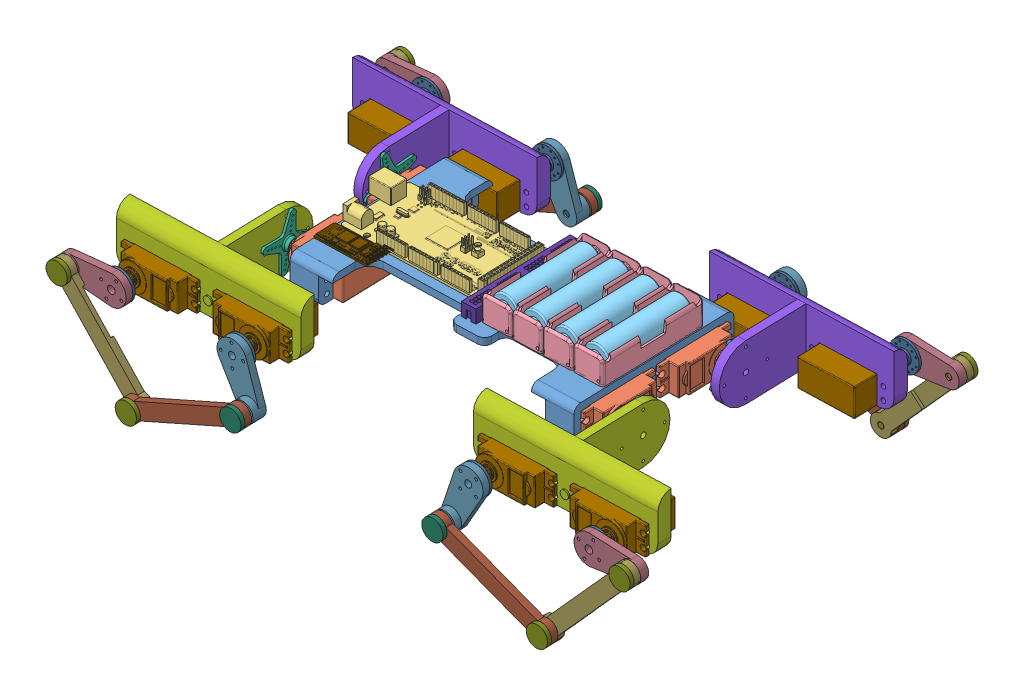
SolidWorks assembly ASSY ver2, configuration Default. Lengths in mm.
Overall size (425.5 115.91 279.7).
69 component instances, 18 part files, 65 mates.
Components (placement in the parent):
- part1 ver2-1: part1 ver2 [Default] at (59.8447 302.7689 135.5904) x (0.999539 0 -0.030355) z (0.030355 0 0.999539) size (275.35 25 175.64)
- Servo MG996R-1: Servo MG996R [Predeterminado] at (-14.9876 282.7689 89.5407) x (0.030355 0 0.999539) z (0 -1 0) size (53.6 47.6 20)
- Servo MG996R-2: Servo MG996R [Predeterminado] at (-12.0493 302.7689 186.2961) x (-0.030355 0 -0.999539) z (0 1 0) size (53.6 47.6 20)
- Servo MG996R-3: Servo MG996R [Predeterminado] at (131.7447 302.7689 85.0846) x (0.030355 0 0.999539) z (0 1 0) size (53.6 47.6 20)
- Servo MG996R-4: Servo MG996R [Predeterminado] at (134.6831 282.7689 181.84) x (-0.030355 0 -0.999539) z (0 -1 0) size (53.6 47.6 20)
- Arduino Mega.step-1: Arduino Mega.step [Default] at (48.5771 307.7689 103.4252) x (-0.949642 0 -0.313338) z (0.313338 0 -0.949642) size (114.59 14.37 81.93)
  - ARDUINO MEGA_1.step-1: ARDUINO MEGA_1.step [Default] at origin size (114.59 14.37 81.93)
- 18650BatteryCase v6.step-1: 18650BatteryCase v6.step [Default] at (136.3002 307.7689 94.7507) x (0.030355 0 0.999539) z (0 1 0) size (76.1 23.18 18.4)
- 18650 battery-1: 18650 battery [Default] at (147.2426 317.7506 100.9214) x (0.302277 -0.953176 -0.00918) z (-0.952737 -0.302416 0.028934) size (18.4 65 18.4)
- 18650 battery-2: 18650 battery [Default] at (125.7525 317.7506 101.5741) x (-0.302277 -0.953176 0.00918) z (-0.952737 0.302416 0.028934) size (18.4 65 18.4)
- 18650BatteryCase v6.step-3: 18650BatteryCase v6.step [Default] at (114.8101 307.7689 95.4034) x (0.030355 0 0.999539) z (0 1 0) size (76.1 23.18 18.4)
- Servo Control Horns-1: Servo Control Horns [4 Arm] at (-59.8704 282.7148 179.7388) x (0.005905 -0.980893 0.194459) z (-0.999539 0 0.030355) size (39 39 5.5)
- Servo Control Horns-2: Servo Control Horns [4 Arm] at (-61.9613 290.1539 110.8872) x (0.02935 -0.255117 0.966465) z (-0.999539 0 0.030355) size (39 39 5.5)
- part2L ver2-1: part2L ver2 [Default] at (-64.6787 292.7689 177.8897) x (0.030355 0 0.999539) z (-0.999539 0 0.030355) size (76 40 130)
- part2R ver2-1: part2R ver2 [Default] at (-67.01 292.7689 101.1251) x (-0.030355 0 -0.999539) z (-0.999539 0 0.030355) size (75 40 130)
- Servo MG996R.step-1: Servo MG996R.step [Default] at (-15.3962 272.7689 71.1446) x (-0.999539 0 0.030355) z (0 -1 0) size (53.62 47.6 20.01)
- Servo MG996R.step-2: Servo MG996R.step [Default] at (-120.6477 292.7689 74.341) x (0.999539 0 -0.030355) z (0 1 0) size (53.62 47.6 20.01)
- Servo MG996R.step-3: Servo MG996R.step [Default] at (-11.3408 292.7689 204.683) x (-0.999539 0 0.030355) z (0 1 0) size (53.62 47.6 20.01)
- Servo MG996R.step-4: Servo MG996R.step [Default] at (-116.2924 272.7689 207.8703) x (0.999539 0 -0.030355) z (0 -1 0) size (53.62 47.6 20.01)
- Circle.step-1: Circle.step [Default] at (-95.6277 278.3089 254.8647) x (0.899955 -0.435126 -0.027331) z (0.030355 0 0.999539) size (21 21 5.5)
- Circle.step-2: Circle.step [Default] at (-9.6532 283.151 252.2537) x (0.998844 0.037283 -0.030334) z (0.030355 0 0.999539) size (21 21 5.5)
- Circle.step-3: Circle.step [Default] at (-105.2045 275.1909 26.0499) x (0.67305 -0.739314 -0.02044) z (-0.030355 0 -0.999539) size (21 21 5.5)
- Circle.step-4: Circle.step [Default] at (-19.4998 289.9232 23.6473) x (0.715779 0.697988 -0.021737) z (-0.030355 0 -0.999539) size (21 21 5.5)
- legpart1 ver2-1: legpart1 ver2 [Default] at (-80.8662 223.9796 272.1746) x (0.919729 0.391558 -0.027931) z (-0.030355 0 -0.999539) size (95 15 5)
- legpart2 ver2-1: legpart2 ver2 [Default] at (-134.5941 283.5044 263.8016) x (0.667805 -0.74406 -0.02028) z (0.030355 0 0.999539) size (95 15 10)
- legpart3 ver2-1: legpart3 ver2 [Default] at (-104.799 282.7689 256.894) x (-0.999239 0.024517 0.030346) z (0.030355 0 0.999539) size (48 21 10)
- legpart4 ver2-1: legpart4 ver2 [Default] at (-19.8382 282.7689 254.3138) x (0.402157 -0.915489 -0.012213) z (0.030355 0 0.999539) size (48 21 15.1)
- legpart3 ver2-2: legpart3 ver2 [Default] at (-111.8565 282.7689 24.5011) x (-0.999239 0.024517 0.030346) z (-0.030355 0 -0.999539) size (48 21 10)
- legpart2 ver2-2: legpart2 ver2 [Default] at (-142.0158 283.5044 19.4143) x (0.667805 -0.74406 -0.02028) z (-0.030355 0 -0.999539) size (95 15 10)
- legpart1 ver2-2: legpart1 ver2 [Default] at (-88.7432 223.9796 12.7941) x (0.919729 0.391558 -0.027931) z (-0.030355 0 -0.999539) size (95 15 5)
- legpart4 ver2-2: legpart4 ver2 [Default] at (-26.8957 282.7689 21.921) x (0.402157 -0.915489 -0.012213) z (-0.030355 0 -0.999539) size (48 21 15.1)
- legpart3 ver2-3: legpart3 ver2 [Default] at (231.5459 282.7689 246.6796) x (0.999239 0.024517 -0.030346) z (0.030355 0 0.999539) size (48 21 10)
- legpart2 ver2-3: legpart2 ver2 [Default] at (261.7052 283.5044 251.7665) x (-0.667805 -0.74406 0.02028) z (0.030355 0 0.999539) size (95 15 10)
- legpart1 ver2-3: legpart1 ver2 [Default] at (208.4326 223.9796 258.3866) x (-0.919729 0.391558 0.027931) z (0.030355 0 0.999539) size (95 15 5)
- legpart4 ver2-3: legpart4 ver2 [Default] at (146.5851 282.7689 249.2598) x (-0.402157 -0.915489 0.012213) z (0.030355 0 0.999539) size (48 21 15.1)
- legpart4 ver2-4: legpart4 ver2 [Default] at (139.5276 282.7689 16.8669) x (-0.402157 -0.915489 0.012213) z (-0.030355 0 -0.999539) size (48 21 15.1)
- legpart1 ver2-4: legpart1 ver2 [Default] at (200.5555 223.9796 -0.9938) x (-0.919729 0.391558 0.027931) z (0.030355 0 0.999539) size (95 15 5)
- legpart2 ver2-4: legpart2 ver2 [Default] at (254.2834 283.5044 7.3791) x (-0.667805 -0.74406 0.02028) z (-0.030355 0 -0.999539) size (95 15 10)
- legpart3 ver2-4: legpart3 ver2 [Default] at (224.4884 282.7689 14.2867) x (0.999239 0.024517 -0.030346) z (-0.030355 0 -0.999539) size (48 21 10)
- legpart5 ver2-1: legpart5 ver2 [Default] at (-7.1967 255.3042 272.9387) x (-0.975892 -0.216232 0.029637) z (0.216132 -0.976342 -0.006564) size (15 18 15)
- legpart6 ver2-1: legpart6 ver2 [Default] at (-80.7751 223.9796 275.1732) x (-0.203537 0.979048 0.006181) z (-0.978597 -0.203631 0.029719) size (15 13 15)
- legpart6 ver2-2: legpart6 ver2 [Default] at (-134.3512 283.5044 271.7979) x (0.979152 0.200942 -0.029736) z (-0.200849 0.979603 0.0061) size (15 13 15)
- legpart6 ver2-3: legpart6 ver2 [Default] at (-142.2587 283.5044 11.418) x (0.979152 0.200942 -0.029736) z (0.200849 -0.979603 -0.0061) size (15 13 15)
- legpart6 ver2-4: legpart6 ver2 [Default] at (-88.9861 223.9796 4.7978) x (-0.203537 0.979048 0.006181) z (0.978597 0.203631 -0.029719) size (15 13 15)
- legpart5 ver2-2: legpart5 ver2 [Default] at (-15.4077 255.3042 2.5633) x (-0.975892 -0.216232 0.029637) z (-0.216132 0.976342 0.006564) size (15 18 15)
- part2L ver2-3: part2L ver2 [Default] at (186.7054 292.7689 170.2555) x (0.030355 0 0.999539) z (-0.999539 0 0.030355) size (76 40 130)
- part2R ver2-3: part2R ver2 [Default] at (184.3741 292.7689 93.4909) x (-0.030355 0 -0.999539) z (-0.999539 0 0.030355) size (75 40 130)
- Servo MG996R.step-9: Servo MG996R.step [Default] at (135.0917 272.7689 200.236) x (0.999539 0 -0.030355) z (0 -1 0) size (53.62 47.6 20.01)
- Servo MG996R.step-10: Servo MG996R.step [Default] at (240.0433 292.7689 197.0488) x (-0.999539 0 0.030355) z (0 1 0) size (53.62 47.6 20.01)
- Servo MG996R.step-11: Servo MG996R.step [Default] at (236.2877 272.7689 63.5012) x (-0.999539 0 0.030355) z (0 -1 0) size (53.62 47.6 20.01)
- Servo MG996R.step-12: Servo MG996R.step [Default] at (131.0363 292.7689 66.6976) x (0.999539 0 -0.030355) z (0 1 0) size (53.62 47.6 20.01)
- Circle.step-9: Circle.step [Default] at (156.7701 282.3867 247.1996) x (0.998844 -0.037283 -0.030334) z (0.030355 0 0.999539) size (21 21 5.5)
- Circle.step-10: Circle.step [Default] at (240.7173 287.2289 244.6503) x (0.899955 0.435126 -0.027331) z (0.030355 0 0.999539) size (21 21 5.5)
- Circle.step-11: Circle.step [Default] at (231.7401 290.3468 15.8173) x (0.67305 0.739314 -0.02044) z (-0.030355 0 -0.999539) size (21 21 5.5)
- Circle.step-12: Circle.step [Default] at (146.9235 275.6145 18.5932) x (0.715779 -0.697988 -0.021737) z (-0.030355 0 -0.999539) size (21 21 5.5)
- legpart6 ver2-5: legpart6 ver2 [Default] at (261.948 283.5044 259.7628) x (-0.979152 0.200942 0.029736) z (-0.200849 -0.979603 0.0061) size (15 13 15)
- legpart6 ver2-6: legpart6 ver2 [Default] at (208.6754 223.9796 266.3829) x (0.203537 0.979048 -0.006181) z (-0.978597 0.203631 0.029719) size (15 13 15)
- legpart5 ver2-3: legpart5 ver2 [Default] at (135.0971 255.3042 268.6174) x (0.975892 -0.216232 -0.029637) z (0.216132 0.976342 -0.006564) size (15 18 15)
- legpart5 ver2-4: legpart5 ver2 [Default] at (126.8861 255.3042 -1.758) x (0.975892 -0.216232 -0.029637) z (-0.216132 -0.976342 0.006564) size (15 18 15)
- legpart6 ver2-7: legpart6 ver2 [Default] at (200.4645 223.9796 -3.9924) x (0.203537 0.979048 -0.006181) z (0.978597 -0.203631 -0.029719) size (15 13 15)
- legpart6 ver2-8: legpart6 ver2 [Default] at (254.0406 283.5044 -0.6172) x (-0.979152 0.200942 0.029736) z (0.200849 0.979603 -0.0061) size (15 13 15)
- breadboard power rail-1: breadboard power rail [Default] at (67.9319 307.7689 135.7049) x (0.999539 0 -0.030355) z (0.030355 0 0.999539) size (11.75 9.53 82.87)
- 18650BatteryCase v6.step-4: 18650BatteryCase v6.step [Default] at (117.1171 307.7689 171.3684) x (-0.030355 0 -0.999539) z (0 1 0) size (76.1 23.18 18.4)
- 18650BatteryCase v6.step-5: 18650BatteryCase v6.step [Default] at (95.627 307.7689 172.021) x (-0.030355 0 -0.999539) z (0 1 0) size (76.1 23.18 18.4)
- 18650 battery-3: 18650 battery [Default] at (104.2624 317.7506 102.2267) x (0.302277 -0.953176 -0.00918) z (-0.952737 -0.302416 0.028934) size (18.4 65 18.4)
- 18650 battery-4: 18650 battery [Default] at (82.7723 317.7506 102.8793) x (-0.302277 -0.953176 0.00918) z (-0.952737 0.302416 0.028934) size (18.4 65 18.4)
- HC-05-1: HC-05 [Default] at (-20.5857 307.7589 172.0486) x (0.999539 0 -0.030355) z (0.030355 0 0.999539) size (42.58 6.55 16)
- Servo Control Horns-3: Servo Control Horns [4 Arm] at (179.3255 295.3838 83.7289) x (-0.02935 0.255117 -0.966465) z (0.999539 0 -0.030355) size (39 39 5.5)
- Servo Control Horns-4: Servo Control Horns [4 Arm] at (181.8971 302.823 168.4065) x (-0.005905 0.980893 -0.194459) z (0.999539 0 -0.030355) size (39 39 5.5)
Mates (geometry in assembly coordinates):
- 일치1: coincident: plane of part1 ver2-1 through (59.8447 302.7689 135.5904) normal (0 -1 0); plane of Servo MG996R-2 through (-48.6324 302.7689 187.4071) normal (0 1 0)
- 거리1: distance = 0.5 mm: plane of Servo MG996R-2 through (-48.6324 302.7689 187.4071) normal (0.030355 0 0.999539); plane of part1 ver2-1 through (61.3321 282.7689 184.5678) normal (-0.030355 0 -0.999539)
- 일치2: coincident: plane of part1 ver2-1 through (59.8447 302.7689 135.5904) normal (0 -1 0); plane of Servo MG996R-1 through (-51.5708 302.7689 90.6517) normal (0 1 0)
- 거리2: distance = 0.5 mm: plane of Servo MG996R-1 through (-50.3475 282.7689 130.9331) normal (0.030355 0 0.999539); plane of part1 ver2-1 through (59.617 282.7689 128.0938) normal (-0.030355 0 -0.999539)
- 일치3: coincident: plane of part1 ver2-1 through (-41.9305 307.7689 78.6535) normal (-0.999539 0 0.030355); plane of Servo MG996R-2 through (-38.4352 302.7689 193.7504) normal (0.999539 0 -0.030355)
- 일치4: coincident: plane of part1 ver2-1 through (-41.9305 307.7689 78.6535) normal (-0.999539 0 0.030355); plane of Servo MG996R-1 through (-40.1502 282.7689 137.2765) normal (0.999539 0 -0.030355)
- 일치10: coincident: plane of part1 ver2-1 through (59.8447 307.7689 135.5904) normal (0 1 0); plane of 18650BatteryCase v6.step-1 through (148.1988 307.7689 132.4069) normal (0 -1 0)
- 동심1: concentric: cylinder of 18650BatteryCase v6.step-1 through (149.3067 317.7506 168.8901) axis (-0.030355 0 -0.999539) radius 4.5; cylinder of 18650 battery-1 through (149.1549 317.7506 163.8924) axis (-0.030355 0 -0.999539) radius 9.2
- 거리3: distance = 5 mm: plane of 18650 battery-1 through (147.2426 317.7506 100.9214) normal (-0.030355 0 -0.999539); plane of 18650BatteryCase v6.step-1 through (137.8451 307.7689 96.2045) normal (0.030355 0 0.999539)
- 거리4: distance = 22.5 mm: plane of part1 ver2-1 through (131.6337 307.7689 193.4379) normal (0.030355 0 0.999539); plane of 18650BatteryCase v6.step-1 through (138.6072 307.7689 170.7157) normal (0.030355 0 0.999539)
- 일치15: coincident: plane of Servo MG996R-2 through (-59.9309 292.7689 177.7456) normal (-0.999539 0 0.030355); plane of Servo Control Horns-1 through (-59.8704 282.7148 179.7388) normal (0.999539 0 -0.030355)
- 동심2: concentric: cylinder of Servo MG996R-2 through (-53.0341 292.7689 177.5361) axis (-0.999539 0 0.030355) radius 1.3; cylinder of Servo Control Horns-1 through (-61.6801 292.7689 177.7987) axis (0.999539 0 -0.030355) radius 1.25
- 일치16: coincident: plane of Servo MG996R-1 through (-62.2621 292.7689 100.981) normal (-0.999539 0 0.030355); plane of Servo Control Horns-2 through (-61.9613 290.1539 110.8872) normal (0.999539 0 -0.030355)
- 동심3: concentric: cylinder of Servo MG996R-1 through (-55.3653 292.7689 100.7715) axis (-0.999539 0 0.030355) radius 1.3; cylinder of Servo Control Horns-2 through (-64.0113 292.7689 101.0341) axis (0.999539 0 -0.030355) radius 1.25
- 일치17: coincident: plane of Servo Control Horns-2 through (-63.7105 290.1539 110.9403) normal (-0.999539 0 0.030355); plane of part2R ver2-1 through (-64.0113 292.7689 101.0341) normal (0.999539 0 -0.030355)
- 동심4: concentric: cylinder of Servo Control Horns-2 through (-64.0113 292.7689 101.0341) axis (0.999539 0 -0.030355) radius 1.25; cylinder of part2R ver2-1 through (-64.0113 292.7689 101.0341) axis (-0.999539 0 0.030355) radius 2
- 일치18: coincident: plane of Servo Control Horns-1 through (-61.6196 282.7148 179.7919) normal (-0.999539 0 0.030355); plane of part2L ver2-1 through (-61.6801 292.7689 177.7987) normal (0.999539 0 -0.030355)
- 동심5: concentric: cylinder of Servo Control Horns-1 through (-61.6801 292.7689 177.7987) axis (0.999539 0 -0.030355) radius 1.25; cylinder of part2L ver2-1 through (-61.6801 292.7689 177.7987) axis (-0.999539 0 0.030355) radius 2
- 일치19: coincident: plane of part2R ver2-1 through (-68.6795 292.7689 46.1505) normal (-0.030355 0 -0.999539); plane of Servo MG996R.step-2 through (-128.1021 292.7689 47.9551) normal (0.030355 0 0.999539)
- 일치20: coincident: plane of part2R ver2-1 through (-68.6795 292.7689 46.1505) normal (-0.030355 0 -0.999539); plane of Servo MG996R.step-1 through (-9.5567 272.7689 44.355) normal (0.030355 0 0.999539)
- 일치22: coincident: plane of part2R ver2-1 through (-121.3515 292.7689 57.7547) normal (0 -1 0); plane of Servo MG996R.step-2 through (-121.7587 292.7689 37.7578) normal (0 1 0)
- 일치23: coincident: plane of part2R ver2-1 through (-15.4004 292.7689 54.5371) normal (0 -1 0); plane of Servo MG996R.step-1 through (-16.5072 292.7689 34.5615) normal (0 1 0)
- 거리6: distance = 0.5 mm: plane of Servo MG996R.step-1 through (-16.5072 272.7689 34.5615) normal (0.999539 0 -0.030355); plane of part2R ver2-1 through (-15.4004 292.7689 54.5371) normal (-0.999539 0 0.030355)
- 거리7: distance = 0.5 mm: plane of part2R ver2-1 through (-80.3704 292.7689 56.5101) normal (-0.999539 0 0.030355); plane of Servo MG996R.step-2 through (-81.4773 292.7689 36.5345) normal (0.999539 0 -0.030355)
- 일치24: coincident: plane of part2L ver2-1 through (-10.3372 292.7689 221.2602) normal (0 -1 0); plane of Servo MG996R.step-3 through (-10.2298 292.7689 241.2662) normal (0 1 0)
- 일치25: coincident: plane of part2L ver2-1 through (-116.2883 292.7689 224.4778) normal (0 -1 0); plane of Servo MG996R.step-4 through (-115.1814 292.7689 244.4534) normal (0 1 0)
- 일치26: coincident: plane of part2L ver2-1 through (-63.0092 292.7689 232.8644) normal (0.030355 0 0.999539); plane of Servo MG996R.step-4 through (-122.1319 272.7689 234.6599) normal (-0.030355 0 -0.999539)
- 일치27: coincident: plane of part2L ver2-1 through (-63.0092 292.7689 232.8644) normal (0.030355 0 0.999539); plane of Servo MG996R.step-3 through (-57.4617 292.7689 232.6959) normal (-0.030355 0 -0.999539)
- 거리8: distance = 0.5 mm: plane of Servo MG996R.step-4 through (-115.1814 272.7689 244.4534) normal (-0.999539 0 0.030355); plane of part2L ver2-1 through (-116.2883 272.7689 224.4778) normal (0.999539 0 -0.030355)
- 거리9: distance = 0.5 mm: plane of Servo MG996R.step-3 through (-10.2298 292.7689 241.2662) normal (0.999539 0 -0.030355); plane of part2L ver2-1 through (-10.3372 272.7689 221.2602) normal (-0.999539 0 0.030355)
- 일치28: coincident: plane of Servo MG996R.step-4 through (-104.8522 282.7689 255.1448) normal (0.030355 0 0.999539); plane of Circle.step-1 through (-95.6277 278.3089 254.8647) normal (-0.030355 0 -0.999539)
- 동심7: concentric: cylinder of Servo MG996R.step-4 through (-105.0616 282.7689 248.248) axis (0.030355 0 0.999539) radius 1.3; cylinder of Circle.step-1 through (-104.799 282.7689 256.894) axis (-0.030355 0 -0.999539) radius 1.25
- 일치30: coincident: plane of Servo MG996R.step-3 through (-19.8913 282.7689 252.5646) normal (0.030355 0 0.999539); plane of Circle.step-2 through (-9.6532 283.151 252.2537) normal (-0.030355 0 -0.999539)
- 동심8: concentric: cylinder of Servo MG996R.step-3 through (-20.1008 282.7689 245.6678) axis (0.030355 0 0.999539) radius 1.3; cylinder of Circle.step-2 through (-19.8382 282.7689 254.3138) axis (-0.030355 0 -0.999539) radius 1.25
- 동심9: concentric: cylinder of Servo MG996R.step-2 through (-111.8878 282.7689 33.3562) axis (-0.030355 0 -0.999539) radius 1.3; cylinder of Circle.step-3 through (-112.1564 282.7689 24.5102) axis (0.030355 0 0.999539) radius 1.25
- 일치32: coincident: plane of Servo MG996R.step-1 through (-26.8365 282.7689 23.8701) normal (-0.030355 0 -0.999539); plane of Circle.step-4 through (-19.4998 289.9232 23.6473) normal (0.030355 0 0.999539)
- 동심10: concentric: cylinder of Servo MG996R.step-1 through (-26.6271 282.7689 30.7669) axis (-0.030355 0 -0.999539) radius 1.3; cylinder of Circle.step-4 through (-26.8896 282.7689 22.1209) axis (0.030355 0 0.999539) radius 1.25
- 일치33: coincident: plane of Circle.step-1 through (-104.799 282.7689 256.894) normal (0.030355 0 0.999539); plane of legpart3 ver2-1 through (-104.799 282.7689 256.894) normal (-0.030355 0 -0.999539)
- 동심11: concentric: cylinder of Circle.step-1 through (-104.799 282.7689 256.894) axis (-0.030355 0 -0.999539) radius 1.25; cylinder of legpart3 ver2-1 through (-104.6473 282.7689 261.8917) axis (-0.030355 0 -0.999539) radius 2.75
- 동심12: concentric: cylinder of legpart2 ver2-1 through (-134.4423 283.5044 268.7993) axis (-0.030355 0 -0.999539) radius 4.5; cylinder of legpart3 ver2-1 through (-134.4726 283.5044 267.7998) axis (-0.030355 0 -0.999539) radius 4.25
- 일치35: coincident: plane of legpart1 ver2-1 through (-81.0179 223.9796 267.1769) normal (-0.030355 0 -0.999539); plane of legpart2 ver2-1 through (-134.4423 283.5044 268.7993) normal (0.030355 0 0.999539)
- 동심13: concentric: cylinder of legpart1 ver2-1 through (-81.0179 223.9796 267.1769) axis (0.030355 0 0.999539) radius 4.5; cylinder of legpart2 ver2-1 through (-81.4125 223.9796 254.1829) axis (0.030355 0 0.999539) radius 2.25
- 일치36: coincident: plane of Circle.step-2 through (-19.8382 282.7689 254.3138) normal (0.030355 0 0.999539); plane of legpart4 ver2-1 through (-19.8382 282.7689 254.3138) normal (-0.030355 0 -0.999539)
- 동심14: concentric: cylinder of Circle.step-2 through (-19.8382 282.7689 254.3138) axis (-0.030355 0 -0.999539) radius 1.25; cylinder of legpart4 ver2-1 through (-19.6864 282.7689 259.3115) axis (-0.030355 0 -0.999539) radius 2.5
- 동심15: concentric: cylinder of legpart1 ver2-1 through (-7.4396 255.3042 264.9424) axis (0.030355 0 0.999539) radius 4.5; cylinder of legpart4 ver2-1 through (-7.3151 255.3042 269.0405) axis (-0.030355 0 -0.999539) radius 4.25
- 일치37: coincident: plane of legpart2 ver2-1 through (-134.5941 283.5044 263.8016) normal (-0.030355 0 -0.999539); plane of legpart3 ver2-1 through (-134.5941 283.5044 263.8016) normal (0.030355 0 0.999539)
- 일치39: coincident: plane of Circle.step-3 through (-112.1564 282.7689 24.5102) normal (-0.030355 0 -0.999539); plane of legpart3 ver2-2 through (-111.8565 282.7689 24.5011) normal (0.030355 0 0.999539)
- 동심18: concentric: cylinder of legpart3 ver2-1 through (-135.6868 283.5044 227.8182) axis (0.030355 0 0.999539) radius 2.25; cylinder of legpart6 ver2-2 through (-134.7458 283.5044 258.8039) axis (0.030355 0 0.999539) radius 2.0625
- 일치40: coincident: plane of legpart2 ver2-1 through (-134.4423 283.5044 268.7993) normal (0.030355 0 0.999539); plane of legpart6 ver2-2 through (-134.4423 283.5044 268.7993) normal (-0.030355 0 -0.999539)
- 동심19: concentric: cylinder of legpart4 ver2-1 through (-8.4109 255.3042 232.9571) axis (0.030355 0 0.999539) radius 2.25; cylinder of legpart5 ver2-1 through (-7.7431 255.3042 254.947) axis (0.030355 0 0.999539) radius 2.0625
- 일치41: coincident: plane of legpart1 ver2-1 through (-80.8662 223.9796 272.1746) normal (0.030355 0 0.999539); plane of legpart5 ver2-1 through (-7.2878 255.3042 269.9401) normal (-0.030355 0 -0.999539)
- 동심20: concentric: cylinder of legpart2 ver2-1 through (-81.4125 223.9796 254.1829) axis (0.030355 0 0.999539) radius 2.25; cylinder of legpart6 ver2-1 through (-81.1697 223.9796 262.1792) axis (0.030355 0 0.999539) radius 2.0625
- 일치42: coincident: plane of legpart1 ver2-1 through (-80.8662 223.9796 272.1746) normal (0.030355 0 0.999539); plane of legpart6 ver2-1 through (-80.8662 223.9796 272.1746) normal (-0.030355 0 -0.999539)
- 거리12: distance = 7 mm: plane of part1 ver2-1 through (-11.1248 307.7689 104.7304) normal (-0.030355 0 -0.999539); plane of Arduino Mega.step-1/ARDUINO MEGA_1.step-1 through (11.4025 307.7689 111.0495) normal (-0.030355 0 -0.999539)
- 일치43: coincident: plane of part1 ver2-1 through (59.8447 307.7689 135.5904) normal (0 1 0); plane of Arduino Mega.step-1/ARDUINO MEGA_1.step-1 through (-37.1106 307.7689 138.5348) normal (0 -1 0)
- 일치45: coincident: plane of part1 ver2-1 through (59.8447 307.7689 135.5904) normal (0 1 0); plane of breadboard power rail-1 through (64.0879 307.7689 176.4804) normal (0 -1 0)
- 거리15: distance = 8 mm: plane of part1 ver2-1 through (-9.1213 307.7689 170.7) normal (0.030355 0 0.999539); plane of breadboard power rail-1 through (64.0879 317.2939 176.4804) normal (0.030355 0 0.999539)
- 일치46: coincident: plane of breadboard power rail-1 through (71.7759 317.2939 94.9295) normal (0.999539 0 -0.030355); plane of 18650BatteryCase v6.step-5 through (71.83 307.7689 96.7086) normal (-0.999539 0 0.030355)
- 거리16: distance = 5 mm: plane of part1 ver2-1 through (-41.9305 307.7689 78.6535) normal (-0.999539 0 0.030355); plane of Arduino Mega.step-1/ARDUINO MEGA_1.step-1 through (-45.4105 310.0689 128.7822) normal (-0.999539 0 0.030355)
- 일치47: coincident: plane of part1 ver2-1 through (59.8447 307.7689 135.5904) normal (0 1 0); plane of HC-05-1 through (-20.5857 307.7689 172.0486) normal (0 -1 0)
- 일치48: coincident: plane of Arduino Mega.step-1/ARDUINO MEGA_1.step-1 through (12.981 307.7689 163.0256) normal (0.030355 0 0.999539); plane of HC-05-1 through (-2.3371 309.0589 163.4907) normal (-0.030355 0 -0.999539)
- 일치49: coincident: plane of part1 ver2-1 through (-41.9305 307.7689 78.6535) normal (-0.999539 0 0.030355); plane of HC-05-1 through (-39.32 309.0589 164.6139) normal (-0.999539 0 0.030355)
- 평행4: parallel: plane of part1 ver2-1 through (59.8447 302.7689 135.5904) normal (0 -1 0); plane of assembly through (0 0 0) normal (0 1 0)
- 일치50: coincident: plane of Arduino Mega.step-1/ARDUINO MEGA_1.step-1 through (62.9947 307.7689 140.4847) normal (0.999539 0 -0.030355); plane of breadboard power rail-1 through (61.6206 317.2939 95.2379) normal (-0.999539 0 0.030355)
- 평행5: parallel: plane of part1 ver2-1 through (59.8447 307.7689 135.5904) normal (0 1 0); plane of part2R ver2-1 through (-64.0113 312.7689 101.0341) normal (0 1 0)
